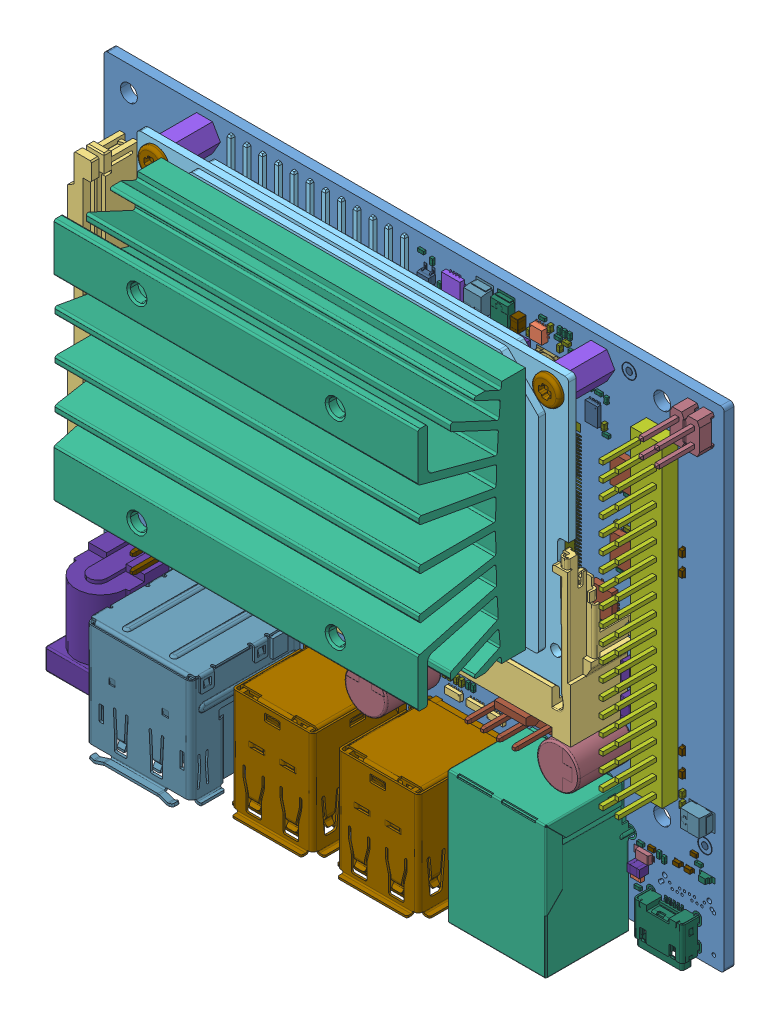
SolidWorks assembly Jetson_Nano_Dev_Kit_3D_b01, configuration Default. Lengths in mm. (continued)
Components (placement in the parent): (continued)
- Jetson_Nano_Dev_Kit_3D_b01(2)^Jetson_Nano_Dev_Kit_3D_b01-1: Jetson_Nano_Dev_Kit_3D_b01(2)^Jetson_Nano_Dev_Kit_3D_b01 [Default] at origin size (100 81.03 30.51) (virtual) (continued)
  - 642-13450_PORG_SYS_BOM^Jetson_Nano_Dev_Kit_3D_b01(2)_Jetson_Nano_Dev_Kit_3D_b01-1: 642-13450_PORG_SYS_BOM^Jetson_Nano_Dev_Kit_3D_b01(2)_Jetson_Nano_Dev_Kit_3D_b01 [Default] at origin size (100 81.03 23.18) (virtual) (continued)
    - 699-13449_PORG_DEV_KIT_PCB_ASSY^642-13450_PORG_SYS_BOM_Jetson_Nano_Dev_Kit_3D_b01(2)_Jetson_Nano_Dev_Kit_3D_b01-1: 699-13449_PORG_DEV_KIT_PCB_ASSY^642-13450_PORG_SYS_BOM_Jetson_Nano_Dev_Kit_3D_b01(2)_Jetson_Nano_Dev_Kit_3D_b01 [Default] at origin size (100 81.03 23.18) (virtual) (continued)
      - 600-13449_PORG_DEV_KIT_PCB_ASSY^699-13449_PORG_DEV_KIT_PCB_ASSY_642-13450_PORG_SYS_BOM_Jetson_Nano_Dev_Kit_3D_b01(2)_Jetson_Nano_Dev_Kit_3D_b01-1: 600-13449_PORG_DEV_KIT_PCB_ASSY^699-13449_PORG_DEV_KIT_PCB_ASSY_642-13450_PORG_SYS_BOM_Jetson_Nano_Dev_Kit_3D_b01(2)_Jetson_Nano_Dev_Kit_3D_b01 [Default] at origin size (100 81.03 23.18) (virtual) (continued)
        - 142-13449-1000-B01-SKU0000^600-13449_PORG_DEV_KIT_PCB_ASSY_699-13449_PORG_DEV_KIT_PCB_ASSY_642-13450_PORG_SYS_BOM_Jetson_Nano_Dev_Kit_3D_b01(2)_Jetson_Nano_Dev_Kit_3D_b01-1: 142-13449-1000-B01-SKU0000^600-13449_PORG_DEV_KIT_PCB_ASSY_699-13449_PORG_DEV_KIT_PCB_ASSY_642-13450_PORG_SYS_BOM_Jetson_Nano_Dev_Kit_3D_b01(2)_Jetson_Nano_Dev_Kit_3D_b01 [Default] at origin size (100 81.03 23.18) (virtual) (continued)
          - 0603_H100^142-13449-1000-B01-SKU0000_600-13449_PORG_DEV_KIT_PCB_ASSY_699-13449_PORG_DEV_KIT_PCB_ASSY_642-13450_PORG_SYS_BOM_Jetson_Nano_Dev_Kit_3D_b01(2)_Jetson_Nano_Dev_Kit_3D_b01-13: 0603_H100^142-13449-1000-B01-SKU0000_600-13449_PORG_DEV_KIT_PCB_ASSY_699-13449_PORG_DEV_KIT_PCB_ASSY_642-13450_PORG_SYS_BOM_Jetson_Nano_Dev_Kit_3D_b01(2)_Jetson_Nano_Dev_Kit_3D_b01 [Default] at (63.9 24.7 1.57) x (0 -1 0) z (0 0 1) size (1.6 0.81 1) (virtual)
          - 080-1669-000_2^142-13449-1000-B01-SKU0000_600-13449_PORG_DEV_KIT_PCB_ASSY_699-13449_PORG_DEV_KIT_PCB_ASSY_642-13450_PORG_SYS_BOM_Jetson_Nano_Dev_Kit_3D_b01(2)_Jetson_Nano_Dev_Kit_3D_b01-1: 080-1669-000_2^142-13449-1000-B01-SKU0000_600-13449_PORG_DEV_KIT_PCB_ASSY_699-13449_PORG_DEV_KIT_PCB_ASSY_642-13450_PORG_SYS_BOM_Jetson_Nano_Dev_Kit_3D_b01(2)_Jetson_Nano_Dev_Kit_3D_b01 [Default] at (0.3 42 1.57) x (0 -1 0) z (0 0 1) size (22.4 5.4 7.7) (virtual)
          - 080-1669-000_2^142-13449-1000-B01-SKU0000_600-13449_PORG_DEV_KIT_PCB_ASSY_699-13449_PORG_DEV_KIT_PCB_ASSY_642-13450_PORG_SYS_BOM_Jetson_Nano_Dev_Kit_3D_b01(2)_Jetson_Nano_Dev_Kit_3D_b01-2: 080-1669-000_2^142-13449-1000-B01-SKU0000_600-13449_PORG_DEV_KIT_PCB_ASSY_699-13449_PORG_DEV_KIT_PCB_ASSY_642-13450_PORG_SYS_BOM_Jetson_Nano_Dev_Kit_3D_b01(2)_Jetson_Nano_Dev_Kit_3D_b01 [Default] at (0.3 18 1.57) x (0 -1 0) z (0 0 1) size (22.4 5.4 7.7) (virtual)
          - 320-0965-000_3^142-13449-1000-B01-SKU0000_600-13449_PORG_DEV_KIT_PCB_ASSY_699-13449_PORG_DEV_KIT_PCB_ASSY_642-13450_PORG_SYS_BOM_Jetson_Nano_Dev_Kit_3D_b01(2)_Jetson_Nano_Dev_Kit_3D_b01-1: 320-0965-000_3^142-13449-1000-B01-SKU0000_600-13449_PORG_DEV_KIT_PCB_ASSY_699-13449_PORG_DEV_KIT_PCB_ASSY_642-13450_PORG_SYS_BOM_Jetson_Nano_Dev_Kit_3D_b01(2)_Jetson_Nano_Dev_Kit_3D_b01 [Default] at (38.776 37.3 1.57) size (6.6 6.6 4.53) (virtual)
    - 699-13448_PORG_MODULE_PCB_ASSY^642-13450_PORG_SYS_BOM_Jetson_Nano_Dev_Kit_3D_b01(2)_Jetson_Nano_Dev_Kit_3D_b01-1: 699-13448_PORG_MODULE_PCB_ASSY^642-13450_PORG_SYS_BOM_Jetson_Nano_Dev_Kit_3D_b01(2)_Jetson_Nano_Dev_Kit_3D_b01 [Default] at (11.2 22.5 8.2662) size (69.6 45 5.7) (virtual)
      - 600-13448_PORG_MODULE_PCB_ASSY^699-13448_PORG_MODULE_PCB_ASSY_642-13450_PORG_SYS_BOM_Jetson_Nano_Dev_Kit_3D_b01(2)_Jetson_Nano_Dev_Kit_3D_b01-1: 600-13448_PORG_MODULE_PCB_ASSY^699-13448_PORG_MODULE_PCB_ASSY_642-13450_PORG_SYS_BOM_Jetson_Nano_Dev_Kit_3D_b01(2)_Jetson_Nano_Dev_Kit_3D_b01 [Default] at origin size (69.6 45 5.7) (virtual)
        - 142-63448-1GEN_A00^600-13448_PORG_MODULE_PCB_ASSY_699-13448_PORG_MODULE_PCB_ASSY_642-13450_PORG_SYS_BOM_Jetson_Nano_Dev_Kit_3D_b01(2)_Jetson_Nano_Dev_Kit_3D_b01-1: 142-63448-1GEN_A00^600-13448_PORG_MODULE_PCB_ASSY_699-13448_PORG_MODULE_PCB_ASSY_642-13450_PORG_SYS_BOM_Jetson_Nano_Dev_Kit_3D_b01(2)_Jetson_Nano_Dev_Kit_3D_b01 [Default] at origin size (69.6 45 5.7) (virtual)
  - 682-13450_PORG_ME_THER_ASSY^Jetson_Nano_Dev_Kit_3D_b01(2)_Jetson_Nano_Dev_Kit_3D_b01-1: 682-13450_PORG_ME_THER_ASSY^Jetson_Nano_Dev_Kit_3D_b01(2)_Jetson_Nano_Dev_Kit_3D_b01 [Default] at origin size (68.74 39.4 29.11) (virtual)
    - PORG_HSK_ASSY^682-13450_PORG_ME_THER_ASSY_Jetson_Nano_Dev_Kit_3D_b01(2)_Jetson_Nano_Dev_Kit_3D_b01-1: PORG_HSK_ASSY^682-13450_PORG_ME_THER_ASSY_Jetson_Nano_Dev_Kit_3D_b01(2)_Jetson_Nano_Dev_Kit_3D_b01 [Default] at (11.2 22.5 12.2762) size (58.7 39.4 17.3) (virtual)
      - 110-0111-000^PORG_HSK_ASSY_682-13450_PORG_ME_THER_ASSY_Jetson_Nano_Dev_Kit_3D_b01(2)_Jetson_Nano_Dev_Kit_3D_b01-1: 110-0111-000^PORG_HSK_ASSY_682-13450_PORG_ME_THER_ASSY_Jetson_Nano_Dev_Kit_3D_b01(2)_Jetson_Nano_Dev_Kit_3D_b01 [Default] at origin size (58.7 39.4 17.3) (virtual)
    - PORG_LEAF_SPRING_DRAWN^682-13450_PORG_ME_THER_ASSY_Jetson_Nano_Dev_Kit_3D_b01(2)_Jetson_Nano_Dev_Kit_3D_b01-1: PORG_LEAF_SPRING_DRAWN^682-13450_PORG_ME_THER_ASSY_Jetson_Nano_Dev_Kit_3D_b01(2)_Jetson_Nano_Dev_Kit_3D_b01 [Default] at (11.2001 22.4999 7.8662) x (1 0.000006 0) z (0 0 1) size (39.83 21.3 0.8) (virtual)
    - 155-0746-000^682-13450_PORG_ME_THER_ASSY_Jetson_Nano_Dev_Kit_3D_b01(2)_Jetson_Nano_Dev_Kit_3D_b01-1: 155-0746-000^682-13450_PORG_ME_THER_ASSY_Jetson_Nano_Dev_Kit_3D_b01(2)_Jetson_Nano_Dev_Kit_3D_b01 [Default] at (12.2 58.5 1.57) size (5.14 4.45 6.57) (virtual)
    - 155-0746-000^682-13450_PORG_ME_THER_ASSY_Jetson_Nano_Dev_Kit_3D_b01(2)_Jetson_Nano_Dev_Kit_3D_b01-2: 155-0746-000^682-13450_PORG_ME_THER_ASSY_Jetson_Nano_Dev_Kit_3D_b01(2)_Jetson_Nano_Dev_Kit_3D_b01 [Default] at (75.8 58.5 1.57) size (5.14 4.45 6.57) (virtual)
    - 155-0754-000^682-13450_PORG_ME_THER_ASSY_Jetson_Nano_Dev_Kit_3D_b01(2)_Jetson_Nano_Dev_Kit_3D_b01-1: 155-0754-000^682-13450_PORG_ME_THER_ASSY_Jetson_Nano_Dev_Kit_3D_b01(2)_Jetson_Nano_Dev_Kit_3D_b01 [Default] at (12.2 58.5 5.7662) x (-1 0 0) z (0 0 -1) size (4.55 4.55 4.53) (virtual)
    - 155-0754-000^682-13450_PORG_ME_THER_ASSY_Jetson_Nano_Dev_Kit_3D_b01(2)_Jetson_Nano_Dev_Kit_3D_b01-2: 155-0754-000^682-13450_PORG_ME_THER_ASSY_Jetson_Nano_Dev_Kit_3D_b01(2)_Jetson_Nano_Dev_Kit_3D_b01 [Default] at (75.8 58.5 5.7662) x (-1 0 0) z (0 0 -1) size (4.55 4.55 4.53) (virtual)
    - 155-0754-000^682-13450_PORG_ME_THER_ASSY_Jetson_Nano_Dev_Kit_3D_b01(2)_Jetson_Nano_Dev_Kit_3D_b01-3: 155-0754-000^682-13450_PORG_ME_THER_ASSY_Jetson_Nano_Dev_Kit_3D_b01(2)_Jetson_Nano_Dev_Kit_3D_b01 [Default] at (12.2 58.5 3.7) size (4.55 4.55 4.53) (virtual)
    - 155-0754-000^682-13450_PORG_ME_THER_ASSY_Jetson_Nano_Dev_Kit_3D_b01(2)_Jetson_Nano_Dev_Kit_3D_b01-4: 155-0754-000^682-13450_PORG_ME_THER_ASSY_Jetson_Nano_Dev_Kit_3D_b01(2)_Jetson_Nano_Dev_Kit_3D_b01 [Default] at (75.8 58.5 3.7) size (4.55 4.55 4.53) (virtual)
    - 155-0717-000^682-13450_PORG_ME_THER_ASSY_Jetson_Nano_Dev_Kit_3D_b01(2)_Jetson_Nano_Dev_Kit_3D_b01-1: 155-0717-000^682-13450_PORG_ME_THER_ASSY_Jetson_Nano_Dev_Kit_3D_b01(2)_Jetson_Nano_Dev_Kit_3D_b01 [Default] at (18.1871 28.4982 13.4762) x (0 0 -1) z (0 1 0) size (6.41 4.7 4.7) (virtual)
    - 155-0717-000^682-13450_PORG_ME_THER_ASSY_Jetson_Nano_Dev_Kit_3D_b01(2)_Jetson_Nano_Dev_Kit_3D_b01-2: 155-0717-000^682-13450_PORG_ME_THER_ASSY_Jetson_Nano_Dev_Kit_3D_b01(2)_Jetson_Nano_Dev_Kit_3D_b01 [Default] at (18.1871 43.4018 13.4762) x (0 0 -1) z (0 1 0) size (6.41 4.7 4.7) (virtual)
    - 155-0717-000^682-13450_PORG_ME_THER_ASSY_Jetson_Nano_Dev_Kit_3D_b01(2)_Jetson_Nano_Dev_Kit_3D_b01-3: 155-0717-000^682-13450_PORG_ME_THER_ASSY_Jetson_Nano_Dev_Kit_3D_b01(2)_Jetson_Nano_Dev_Kit_3D_b01 [Default] at (51.6129 43.4018 13.4762) x (0 0 -1) z (0 1 0) size (6.41 4.7 4.7) (virtual)
    - 155-0717-000^682-13450_PORG_ME_THER_ASSY_Jetson_Nano_Dev_Kit_3D_b01(2)_Jetson_Nano_Dev_Kit_3D_b01-4: 155-0717-000^682-13450_PORG_ME_THER_ASSY_Jetson_Nano_Dev_Kit_3D_b01(2)_Jetson_Nano_Dev_Kit_3D_b01 [Default] at (51.6129 28.4982 13.4762) x (0 0 -1) z (0 1 0) size (6.41 4.7 4.7) (virtual)
